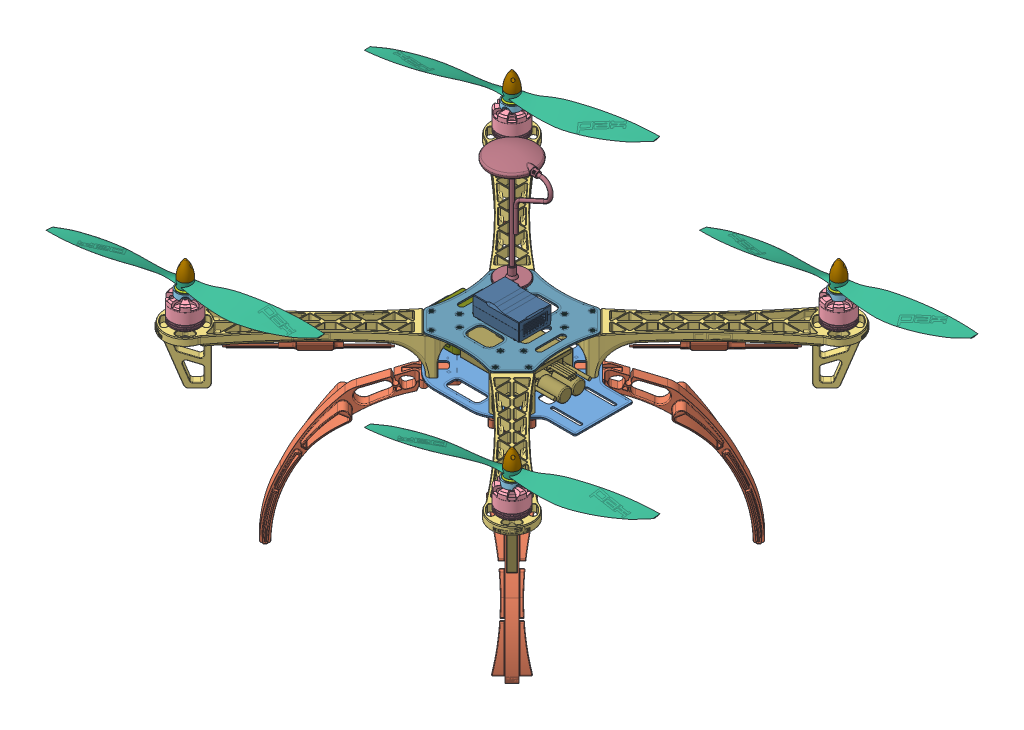
SolidWorks assembly DRON, configuration Default. Lengths in mm.
Overall size (544.72 294.02 417.77).
58 component instances, 16 part files, 61 mates.
Components (placement in the parent):
- Kimi Chasis-1: Kimi Chasis [Default] at origin size (180.5 1.6 116.75)
- Kimi stand-1: Kimi stand [Default] at (35.0931 -4.75 35.0872) x (0.707107 0 -0.707107) z (0.707107 0 0.707107) size (44.27 147.01 143.39)
- Kimi stand-2: Kimi stand [Default] at (35.0872 -4.75 -35.0931) x (-0.707107 0 -0.707107) z (0.707107 0 -0.707107) size (44.27 147.01 143.39)
- Kimi stand-3: Kimi stand [Default] at (-35.0931 -4.75 -35.0872) x (-0.707107 0 0.707107) z (-0.707107 0 -0.707107) size (44.27 147.01 143.39)
- Kimi stand-4: Kimi stand [Default] at (-35.0872 -4.75 35.0931) x (0.707107 0 0.707107) z (-0.707107 0 0.707107) size (44.27 147.01 143.39)
- Kimi DJI arm-1: Kimi DJI arm [Default] at (-159.7001 35.75 -159.7001) x (0.707107 0 0.707107) z (-0.707107 0 0.707107) size (216.5 54.25 40.8)
- Kimi DJI arm-5: Kimi DJI arm [Default] at (-159.7001 35.75 159.7001) x (0.707107 0 -0.707107) z (0.707107 0 0.707107) size (216.5 54.25 40.8)
- Kimi DJI arm-6: Kimi DJI arm [Default] at (159.7001 35.75 -159.7001) x (-0.707107 0 0.707107) z (-0.707107 0 -0.707107) size (216.5 54.25 40.8)
- Kimi DJI arm-7: Kimi DJI arm [Default] at (159.7001 35.75 159.7001) x (-0.707107 0 -0.707107) z (0.707107 0 -0.707107) size (216.5 54.25 40.8)
- Kimi MT2208-18-1: Kimi MT2208-18 [Default] at (159.7001 37.75 159.7001) x (0.707107 0 -0.707107) z (0.707107 0 0.707107) size (27.6 26.86 27.6)
- Kimi PROP ADAPTER MT 2208-18-1: Kimi PROP ADAPTER MT 2208-18 [Default] at (159.7253 65.8 159.7068) x (0.966934 0 -0.255028) z (0.255028 0 0.966934) size (17 19.77 17)
- Kimi propeler 9x4-1: Kimi propeler 9x4 [Default] at (163.7804 73.9589 164.5022) x (-0.052057 0 -0.998644) z (-0.998644 0 0.052057) size (73.5 20.08 221.03)
- Kimi Prop Adapter Washer MT2208-18-2: Kimi Prop Adapter Washer MT2208-18 [Default] at (159.7253 65.8 159.7068) size (14.75 2 14.75)
- Kimi Prop Adapter Nut MT2208-18-1: Kimi Prop Adapter Nut MT2208-18 [Default] at (159.7253 74.4589 159.7068) x (-0.272586 0 0.962132) z (-0.962132 0 -0.272586) size (9.98 3.78 7.93)
- Kimi MT2208-18 spinner-1: Kimi MT2208-18 spinner [Default] at (159.7253 74.4589 159.7068) x (-0.813634 0 -0.581377) z (0.581377 0 -0.813634) size (13 16.17 13)
- Kimi MT2208-18-2: Kimi MT2208-18 [Default] at (159.7001 37.75 -159.7001) x (-0.707107 0 -0.707107) z (0.707107 0 -0.707107) size (27.6 26.86 27.6)
- Kimi PROP ADAPTER MT 2208-18-2: Kimi PROP ADAPTER MT 2208-18 [Default] at (159.7253 65.8 -159.7068) x (-0.966934 0 -0.255028) z (0.255028 0 -0.966934) size (17 19.77 17)
- Kimi propeler 9x4-2: Kimi propeler 9x4 [Default] at (156.1907 73.9589 -164.8979) x (-0.052057 0 0.998644) z (0.998644 0 0.052057) size (73.5 20.08 221.03)
- Kimi Prop Adapter Washer MT2208-18-3: Kimi Prop Adapter Washer MT2208-18 [Default] at (159.7253 65.8 -159.7068) size (14.75 2 14.75)
- Kimi Prop Adapter Nut MT2208-18-2: Kimi Prop Adapter Nut MT2208-18 [Default] at (159.7253 74.4589 -159.7068) x (-0.272586 0 -0.962132) z (0.962132 0 -0.272586) size (9.98 3.78 7.93)
- Kimi MT2208-18 spinner-2: Kimi MT2208-18 spinner [Default] at (159.7253 74.4589 -159.7068) x (-0.813634 0 0.581377) z (-0.581377 0 -0.813634) size (13 16.17 13)
- Kimi MT2208-18-3: Kimi MT2208-18 [Default] at (-159.7001 37.75 159.7001) x (0.707107 0 0.707107) z (-0.707107 0 0.707107) size (27.6 26.86 27.6)
- Kimi PROP ADAPTER MT 2208-18-3: Kimi PROP ADAPTER MT 2208-18 [Default] at (-159.7253 65.8 159.7068) x (0.966934 0 0.255028) z (-0.255028 0 0.966934) size (17 19.77 17)
- Kimi propeler 9x4-3: Kimi propeler 9x4 [Default] at (-156.1907 73.9589 164.8979) x (0.052057 0 -0.998644) z (-0.998644 0 -0.052057) size (73.5 20.08 221.03)
- Kimi Prop Adapter Washer MT2208-18-4: Kimi Prop Adapter Washer MT2208-18 [Default] at (-159.7253 65.8 159.7068) x (-1 0 0) z (0 0 -1) size (14.75 2 14.75)
- Kimi Prop Adapter Nut MT2208-18-3: Kimi Prop Adapter Nut MT2208-18 [Default] at (-159.7253 74.4589 159.7068) x (0.272586 0 0.962132) z (-0.962132 0 0.272586) size (9.98 3.78 7.93)
- Kimi MT2208-18 spinner-3: Kimi MT2208-18 spinner [Default] at (-159.7253 74.4589 159.7068) x (0.813634 0 -0.581377) z (0.581377 0 0.813634) size (13 16.17 13)
- Kimi MT2208-18-4: Kimi MT2208-18 [Default] at (-159.7001 37.75 -159.7001) x (-0.707107 0 0.707107) z (-0.707107 0 -0.707107) size (27.6 26.86 27.6)
- Kimi PROP ADAPTER MT 2208-18-4: Kimi PROP ADAPTER MT 2208-18 [Default] at (-159.7253 65.8 -159.7068) x (-0.966934 0 0.255028) z (-0.255028 0 -0.966934) size (17 19.77 17)
- Kimi propeler 9x4-4: Kimi propeler 9x4 [Default] at (-163.7804 73.9589 -164.5022) x (0.052057 0 0.998644) z (0.998644 0 -0.052057) size (73.5 20.08 221.03)
- Kimi Prop Adapter Washer MT2208-18-5: Kimi Prop Adapter Washer MT2208-18 [Default] at (-159.7253 65.8 -159.7068) x (-1 0 0) z (0 0 -1) size (14.75 2 14.75)
- Kimi Prop Adapter Nut MT2208-18-4: Kimi Prop Adapter Nut MT2208-18 [Default] at (-159.7253 74.4589 -159.7068) x (0.272586 0 -0.962132) z (0.962132 0 0.272586) size (9.98 3.78 7.93)
- Kimi MT2208-18 spinner-4: Kimi MT2208-18 spinner [Default] at (-159.7253 74.4589 -159.7068) x (0.813634 0 0.581377) z (-0.581377 0 0.813634) size (13 16.17 13)
- Kimi fcNaza - MC-1: Kimi fcNaza - MC [Default] at (0 48.35 0) size (45.7 18.6 32)
- Kimi 30A ESCIRAN-1: Kimi 30A ESCIRAN [Default] at (-97.6184 20.908 -115.7157) x (0.707107 0 -0.707107) z (0.707107 0 0.707107) size (28.83 9.95 119.13)
- Kimi 30A ESCIRAN-2: Kimi 30A ESCIRAN [Default] at (115.7157 20.908 -97.6184) x (0.707107 0 0.707107) z (-0.707107 0 0.707107) size (28.83 9.95 119.13)
- Kimi 30A ESCIRAN-3: Kimi 30A ESCIRAN [Default] at (97.6184 20.908 115.7157) x (-0.707107 0 0.707107) z (-0.707107 0 -0.707107) size (28.83 9.95 119.13)
- Kimi 30A ESCIRAN-4: Kimi 30A ESCIRAN [Default] at (-115.7157 20.908 97.6184) x (-0.707107 0 -0.707107) z (0.707107 0 -0.707107) size (28.83 9.95 119.13)
- Kimi fc Naza - PSU-3: Kimi fc Naza - PSU [Default] at (4.5 13.25 0) x (0 0 -1) z (0 -1 0) size (46.2 88 24)
- Kimi fcNaza - GPS-2: Kimi fcNaza - GPS [Default] at (-35.2481 141.25 -35.2778) x (0.997565 0 0.069742) z (-0.069742 0 0.997565) size (65.49 109 46)
- Kimi Top Plate-1: Kimi Top Plate [Default] at (0.0012 37.5 -0.0271) x (0.00002 0 -1) z (1 0 0.00002) size (106.11 11.51 106.11)
- Vijak-1: Vijak [Default] at (31.2916 38.15 -47.5794) x (1 0 0) z (0 -1 0) size (3.3 3.3 6.4)
- Vijak-2: Vijak [Default] at (19.9776 38.15 -31.3162) x (1 0 0) z (0 -1 0) size (3.3 3.3 6.4)
- Vijak-3: Vijak [Default] at (31.2911 38.15 -20.0022) x (1 0 0) z (0 -1 0) size (3.3 3.3 6.4)
- Vijak-4: Vijak [Default] at (47.5547 38.15 -31.3156) x (1 0 0) z (0 -1 0) size (3.3 3.3 6.4)
- Vijak-5: Vijak [Default] at (-31.2916 38.15 -47.5794) x (-1 0 0) z (0 -1 0) size (3.3 3.3 6.4)
- Vijak-6: Vijak [Default] at (-19.9776 38.15 -31.3162) x (-1 0 0) z (0 -1 0) size (3.3 3.3 6.4)
- Vijak-7: Vijak [Default] at (-31.2911 38.15 -20.0022) x (-1 0 0) z (0 -1 0) size (3.3 3.3 6.4)
- Vijak-8: Vijak [Default] at (-47.5547 38.15 -31.3156) x (-1 0 0) z (0 -1 0) size (3.3 3.3 6.4)
- Vijak-9: Vijak [Default] at (31.2916 38.15 47.5794) x (1 0 0) z (0 -1 0) size (3.3 3.3 6.4)
- Vijak-10: Vijak [Default] at (19.9776 38.15 31.3162) x (1 0 0) z (0 -1 0) size (3.3 3.3 6.4)
- Vijak-11: Vijak [Default] at (31.2911 38.15 20.0022) x (1 0 0) z (0 -1 0) size (3.3 3.3 6.4)
- Vijak-12: Vijak [Default] at (47.5547 38.15 31.3156) x (1 0 0) z (0 -1 0) size (3.3 3.3 6.4)
- Vijak-13: Vijak [Default] at (-31.2916 38.15 47.5794) x (-1 0 0) z (0 -1 0) size (3.3 3.3 6.4)
- Vijak-14: Vijak [Default] at (-19.9776 38.15 31.3162) x (-1 0 0) z (0 -1 0) size (3.3 3.3 6.4)
- Vijak-15: Vijak [Default] at (-31.2911 38.15 20.0022) x (-1 0 0) z (0 -1 0) size (3.3 3.3 6.4)
- Vijak-16: Vijak [Default] at (-47.5547 38.15 31.3156) x (-1 0 0) z (0 -1 0) size (3.3 3.3 6.4)
- box2-1: box2 [Default] at (-50.5 0.75 0) x (0 0 1) z (-1 0 0) size (40 22 35)
Mates (geometry in assembly coordinates):
- Concentric1: concentric anti-aligned: cylinder of Kimi Chasis-1 through (46.8458 -0.76 31.9966) axis (0 -1 0) radius 1.625; cylinder of Kimi stand-1 through (46.8458 -2.75 31.9966) axis (0 1 0) radius 1.5
- Concentric2: concentric anti-aligned: cylinder of Kimi Chasis-1 through (31.9966 -0.76 46.8458) axis (0 -1 0) radius 1.625; cylinder of Kimi stand-1 through (31.9966 -2.75 46.8458) axis (0 1 0) radius 1.5
- Coincident1: coincident anti-aligned: plane of Kimi Chasis-1 through (0 -0.75 0) normal (0 -1 0); plane of Kimi stand-1 through (35.0931 -0.75 35.0872) normal (0 1 0)
- Concentric6: concentric anti-aligned: cylinder of Kimi Chasis-1 through (31.9966 -0.76 -46.8458) axis (0 -1 0) radius 1.625; cylinder of Kimi stand-2 through (31.9966 -2.75 -46.8458) axis (0 1 0) radius 1.5
- Concentric7: concentric anti-aligned: cylinder of Kimi Chasis-1 through (46.8458 -0.76 -31.9966) axis (0 -1 0) radius 1.625; cylinder of Kimi stand-2 through (46.8458 -2.75 -31.9966) axis (0 1 0) radius 1.5
- Coincident2: coincident anti-aligned: plane of Kimi Chasis-1 through (0 -0.75 0) normal (0 -1 0); plane of Kimi stand-2 through (35.0872 -0.75 -35.0931) normal (0 1 0)
- Concentric9: concentric anti-aligned: cylinder of Kimi Chasis-1 through (-46.8458 -0.76 -31.9966) axis (0 -1 0) radius 1.625; cylinder of Kimi stand-3 through (-46.8458 -2.75 -31.9966) axis (0 1 0) radius 1.5
- Concentric10: concentric anti-aligned: cylinder of Kimi Chasis-1 through (-31.9966 -0.76 -46.8458) axis (0 -1 0) radius 1.625; cylinder of Kimi stand-3 through (-31.9966 -2.75 -46.8458) axis (0 1 0) radius 1.5
- Coincident3: coincident anti-aligned: plane of Kimi Chasis-1 through (0 -0.75 0) normal (0 -1 0); plane of Kimi stand-3 through (-35.0931 -0.75 -35.0872) normal (0 1 0)
- Concentric11: concentric anti-aligned: cylinder of Kimi Chasis-1 through (-46.8458 -0.76 31.9966) axis (0 -1 0) radius 1.625; cylinder of Kimi stand-4 through (-46.8458 -2.75 31.9966) axis (0 1 0) radius 1.5
- Concentric12: concentric anti-aligned: cylinder of Kimi Chasis-1 through (-31.9966 -0.76 46.8458) axis (0 -1 0) radius 1.625; cylinder of Kimi stand-4 through (-31.9966 -2.75 46.8458) axis (0 1 0) radius 1.5
- Coincident4: coincident anti-aligned: plane of Kimi Chasis-1 through (0 -0.75 0) normal (0 -1 0); plane of Kimi stand-4 through (-35.0872 -0.75 35.0931) normal (0 1 0)
- Concentric13: concentric aligned: cylinder of Kimi Chasis-1 through (-31.9966 -0.76 -46.8458) axis (0 -1 0) radius 1.625; cylinder of Kimi DJI arm-1 through (-31.9966 -1.25 -46.8458) axis (0 -1 0) radius 1.25
- Concentric14: concentric aligned: cylinder of Kimi Chasis-1 through (-46.8458 -0.76 -31.9966) axis (0 -1 0) radius 1.625; cylinder of Kimi DJI arm-1 through (-46.8458 -1.25 -31.9966) axis (0 -1 0) radius 1.25
- Coincident5: coincident anti-aligned: plane of Kimi Chasis-1 through (0 0.75 0) normal (0 1 0); plane of Kimi DJI arm-1 through (-159.7001 0.75 -159.7001) normal (0 -1 0)
- Concentric32: concentric anti-aligned: cylinder of Kimi DJI arm-1 through (-31.2902 15.2145 -19.9493) axis (0 1 0) radius 1.25; cylinder of ? through (-31.2903 36.74 -19.9493) axis (0 -1 0) radius 1.625
- Concentric33: concentric anti-aligned: cylinder of Kimi DJI arm-1 through (-19.9763 15.2145 -31.2628) axis (0 1 0) radius 1.25; cylinder of ? through (-19.9763 36.74 -31.2628) axis (0 -1 0) radius 1.625
- Coincident8: coincident anti-aligned: plane of Kimi DJI arm-1 through (-6.965 36.75 -35.815) normal (0 1 0); plane of ? through (0.0019 36.75 -152.766) normal (0 -1 0)
- Concentric34: concentric aligned: cylinder of Kimi DJI arm-7 through (159.7001 35.75 159.7001) axis (0 1 0) radius 5; cylinder of Kimi MT2208-18-1 through (159.7001 36.45 159.7001) axis (0 1 0) radius 2.8
- Coincident9: coincident anti-aligned: plane of Kimi DJI arm-7 through (135.6921 37.75 167.9934) normal (0 1 0); plane of Kimi MT2208-18-1 through (159.7001 37.75 159.7001) normal (0 -1 0)
- Concentric35: concentric anti-aligned: cylinder of Kimi DJI arm-7 through (169.2001 35.75 159.7001) axis (0 1 0) radius 1.55; cylinder of Kimi MT2208-18-1 through (169.2001 42.75 159.7001) axis (0 -1 0) radius 1.2
- Concentric36: concentric aligned: cylinder of Kimi MT2208-18-1 through (163.7825 46.8 155.6176) axis (0 1 0) radius 0.8586; cylinder of Kimi PROP ADAPTER MT 2208-18-1 through (163.7825 60.3 155.6176) axis (0 1 0) radius 1.065
- Concentric37: concentric aligned: cylinder of Kimi MT2208-18-1 through (154.1233 46.8 158.2058) axis (0 1 0) radius 0.8586; cylinder of Kimi PROP ADAPTER MT 2208-18-1 through (154.1233 60.3 158.2058) axis (0 1 0) radius 1.065
- Coincident10: coincident anti-aligned: plane of Kimi MT2208-18-1 through (159.7001 60.3 159.7001) normal (0 1 0); plane of Kimi PROP ADAPTER MT 2208-18-1 through (159.7253 60.3 159.7068) normal (0 -1 0)
- Concentric38: concentric aligned: cylinder of Kimi PROP ADAPTER MT 2208-18-1 through (159.7253 79.3 159.7068) axis (0 -1 0) radius 2.485; cylinder of Kimi Prop Adapter Washer MT2208-18-2 through (159.7253 67.8 159.7068) axis (0 -1 0) radius 2.55
- Coincident11: coincident anti-aligned: plane of Kimi PROP ADAPTER MT 2208-18-1 through (159.7253 65.8 159.7068) normal (0 1 0); plane of Kimi Prop Adapter Washer MT2208-18-2 through (159.7253 65.8 159.7068) normal (0 -1 0)
- Concentric39: concentric aligned: cylinder of Kimi PROP ADAPTER MT 2208-18-1 through (159.7253 79.3 159.7068) axis (0 -1 0) radius 2.485; cylinder of Kimi propeler 9x4-1 through (159.7253 74.4589 159.7068) axis (0 -1 0) radius 3.15
- Coincident12: coincident: circle of Kimi propeler 9x4-1; cone of Kimi Prop Adapter Washer MT2208-18-2 through (159.7253 67.8 159.7068) axis (0 1 0)
- Concentric40: concentric aligned: cylinder of Kimi PROP ADAPTER MT 2208-18-1 through (159.7253 79.3 159.7068) axis (0 -1 0) radius 2.485; cylinder of Kimi Prop Adapter Nut MT2208-18-1 through (159.7253 78.2389 159.7068) axis (0 -1 0) radius 2.15
- Concentric41: concentric aligned: cylinder of Kimi PROP ADAPTER MT 2208-18-1 through (159.7253 79.3 159.7068) axis (0 -1 0) radius 2.485; cylinder of Kimi Prop Adapter Nut MT2208-18-1 through (159.7253 78.2389 159.7068) axis (0 -1 0) radius 2.15
- Coincident15: coincident anti-aligned: plane of Kimi propeler 9x4-1 through (159.7253 74.4589 159.7068) normal (0 1 0); plane of Kimi Prop Adapter Nut MT2208-18-1 through (158.4773 74.4589 164.1118) normal (0 -1 0)
- Concentric42: concentric anti-aligned: cone of Kimi PROP ADAPTER MT 2208-18-1 through (159.7253 79.3 159.7068) axis (0 1 0); cylinder of Kimi MT2208-18 spinner-1 through (159.7253 78.2589 159.7068) axis (0 -1 0) radius 5.2829
- Coincident16: coincident anti-aligned: plane of Kimi propeler 9x4-1 through (159.7253 74.4589 159.7068) normal (0 1 0); plane of Kimi MT2208-18 spinner-1 through (159.7253 74.4589 159.7068) normal (0 -1 0)
- Coincident17: coincident anti-aligned: plane of ? through (-0.0042 38.25 152.8201) normal (0 1 0); plane of Kimi fcNaza - MC-1 through (0 38.25 0) normal (0 -1 0)
- Coincident19: coincident aligned: plane of Kimi fcNaza - MC-1 through (0 48.35 0) normal (0 0 1); plane of assembly through (0 0 0) normal (0 0 1)
- Coincident20: coincident aligned: plane of Kimi fcNaza - MC-1 through (0 48.35 0) normal (1 0 0); plane of assembly through (0 0 0) normal (1 0 0)
- Coincident21: coincident aligned: plane of Kimi DJI arm-1 through (-159.7001 35.75 -159.7001) normal (-0.707107 0 0.707107); plane of Kimi 30A ESCIRAN-1 through (-106.6671 20.908 -106.6671) normal (-0.707107 0 0.707107)
- Coincident22: coincident anti-aligned: plane of Kimi DJI arm-1 through (-134.1244 26.75 -162.9743) normal (0 -1 0); plane of Kimi 30A ESCIRAN-1 through (-97.6184 26.75 -115.7157) normal (0 1 0)
- Distance1: distance = 75 mm aligned: plane of Kimi 30A ESCIRAN-1 through (-97.6184 20.908 -115.7157) normal (0.707107 0 0.707107); plane of Kimi DJI arm-1 through (-159.7001 35.75 -159.7001) normal (0.707107 0 0.707107)
- Concentric44: concentric aligned: cylinder of ? through (35.2495 48.25 -35.2222) axis (0 -1 0) radius 2.25; cylinder of Kimi fcNaza - GPS-2 through (35.2495 48.25 -35.2222) axis (0 -1 0) radius 2.25
- Coincident29: coincident anti-aligned: plane of ? through (-0.0042 38.25 152.8201) normal (0 1 0); plane of Kimi fcNaza - GPS-2 through (35.2495 38.25 -35.2222) normal (0 -1 0)
- Coincident31: coincident anti-aligned: plane of Kimi Chasis-1 through (0 0 0) normal (0 0 1); plane of Kimi fc Naza - PSU-3
- Concentric47: concentric anti-aligned: cylinder of Kimi DJI arm-7 through (31.2902 15.2145 19.9493) axis (0 1 0) radius 1.25; cylinder of Kimi Top Plate-1 through (31.2903 36.74 19.9493) axis (0 -1 0) radius 1.625
- Concentric48: concentric anti-aligned: cylinder of Kimi DJI arm-7 through (19.9763 15.2145 31.2628) axis (0 1 0) radius 1.25; cylinder of Kimi Top Plate-1 through (19.9763 36.74 31.2628) axis (0 -1 0) radius 1.625
- Coincident32: coincident anti-aligned: plane of Kimi DJI arm-7 through (6.965 36.75 35.815) normal (0 1 0); plane of Kimi Top Plate-1 through (-152.7919 36.75 -0.0301) normal (0 -1 0)
- Coincident33: coincident anti-aligned: plane of Kimi fcNaza - MC-1 through (0 38.25 0) normal (0 -1 0); plane of Kimi Top Plate-1 through (152.7942 38.25 -0.024) normal (0 1 0)
- Concentric49: concentric aligned: cylinder of Kimi fcNaza - GPS-2 through (-35.2481 48.25 -35.2778) axis (0 -1 0) radius 2.25; cylinder of Kimi Top Plate-1 through (-35.2481 48.25 -35.2778) axis (0 -1 0) radius 2.25
- Coincident35: coincident anti-aligned: plane of Kimi fcNaza - GPS-2 through (-35.2481 38.25 -35.2778) normal (0 -1 0); plane of Kimi Top Plate-1 through (152.7942 38.25 -0.024) normal (0 1 0)
- Coincident36: coincident anti-aligned: plane of Kimi Chasis-1 through (0 0.75 0) normal (0 1 0); plane of Kimi fc Naza - PSU-3 through (4.5 0.75 0) normal (0 -1 0)
- Distance2: distance = 10 mm aligned: plane of Kimi fc Naza - PSU-3 through (30 0.75 16) normal (1 0 0); plane of Kimi Chasis-1 through (40 0.76 15.875) normal (1 0 0)
- Concentric50: concentric anti-aligned: cylinder of Kimi Top Plate-1 through (31.2916 36.74 -47.5794) axis (0 -1 0) radius 1.625; cylinder of Vijak-1 through (31.2916 31.75 -47.5794) axis (0 1 0) radius 1.25
- Coincident38: coincident anti-aligned: plane of Kimi DJI arm-6 through (35.815 36.75 -6.965) normal (0 1 0); plane of Vijak-1 through (31.2916 36.75 -47.5794) normal (0 -1 0)
- Coincident39: coincident anti-aligned: plane of Kimi DJI arm-6 through (35.815 36.75 -6.965) normal (0 1 0); plane of Vijak-4 through (47.5547 36.75 -31.3156) normal (0 -1 0)
- Concentric52: concentric anti-aligned: cylinder of Kimi Top Plate-1 through (47.5547 36.74 -31.3156) axis (0 -1 0) radius 1.625; cylinder of Vijak-4 through (47.5547 31.75 -31.3156) axis (0 1 0) radius 1.25
- Coincident40: coincident anti-aligned: plane of Kimi DJI arm-6 through (35.815 36.75 -6.965) normal (0 1 0); plane of Vijak-3 through (31.2911 36.75 -20.0022) normal (0 -1 0)
- Concentric53: concentric anti-aligned: cylinder of Kimi Top Plate-1 through (31.2911 36.74 -20.0022) axis (0 -1 0) radius 1.625; cylinder of Vijak-3 through (31.2911 31.75 -20.0022) axis (0 1 0) radius 1.25
- Coincident41: coincident anti-aligned: plane of Kimi DJI arm-6 through (35.815 36.75 -6.965) normal (0 1 0); plane of Vijak-2 through (19.9776 36.75 -31.3162) normal (0 -1 0)
- Concentric54: concentric anti-aligned: cylinder of Kimi Top Plate-1 through (19.9776 36.74 -31.3162) axis (0 -1 0) radius 1.625; cylinder of Vijak-2 through (19.9776 31.75 -31.3162) axis (0 1 0) radius 1.25
- Coincident43: coincident anti-aligned: plane of Kimi Chasis-1 through (0 0.75 0) normal (0 1 0); plane of box2-1 through (-38 0.75 15) normal (0 -1 0)
- Distance4: distance = 5 mm anti-aligned: plane of Kimi fc Naza - PSU-3 through (-28 3.75 22.5) normal (-1 0 0); plane of box2-1 through (-33 22.75 -15) normal (1 0 0)
- Coincident45: coincident aligned: plane of box2-1 through (-50.5 0.75 0) normal (0 0 1); plane of assembly through (0 0 0) normal (0 0 1)
